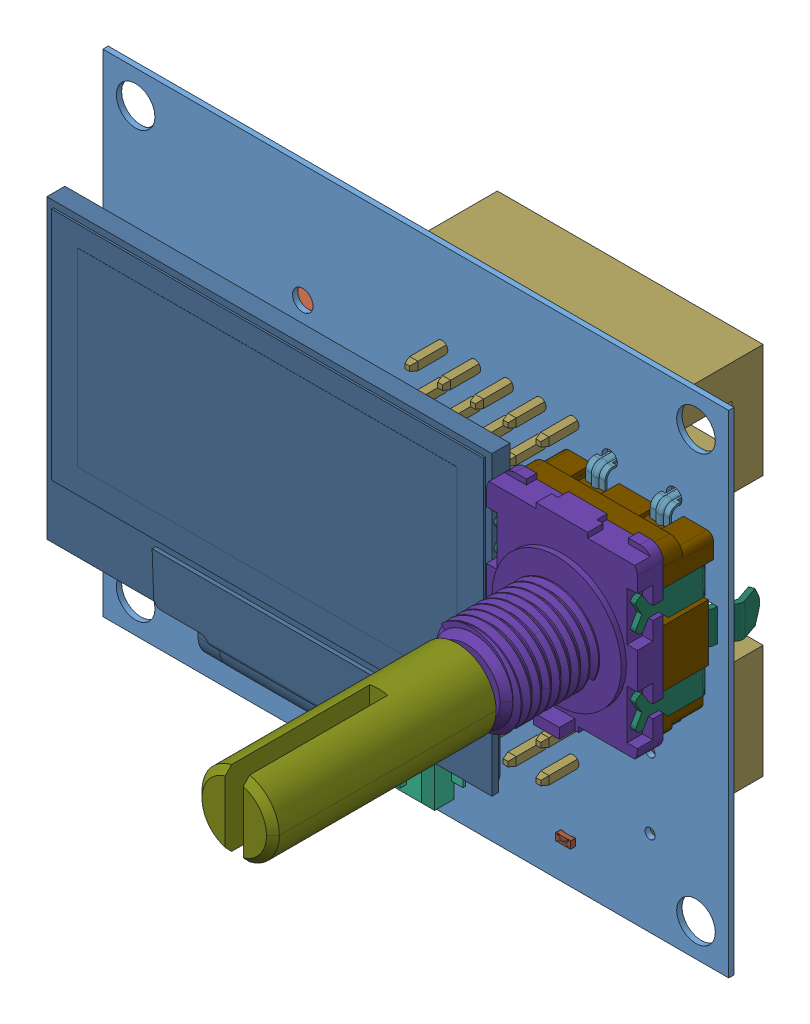
SolidWorks assembly PCB2, configuration 默认. Lengths in mm.
Overall size (48.51 38.1 41.11).
81 component instances, 19 part files, 0 mates.
Components (placement in the parent):
- PCB2.step-1: PCB2.step [默认] at origin size (48.51 38.1 41.11)
  - Board.step-1: Board.step [默认] at origin size (48.51 38.1 0.41)
    - Open CASCADE STEP translator 6.8 1.1.1.step-1: Open CASCADE STEP translator 6.8 1.1.1.step [默认] at (0 0 -0.4115) size (48.51 38.1 0.41)
  - U2.step-1: U2.step [默认] at origin size (18.85 27.3 3.6)
    - User_Library-SDCARD.step-1: User_Library-SDCARD.step [默认] at (12.9551 16.5451 -0.4115) x (0 1 0) z (0 0 -1) size (27.3 18 3)
      - Pad002.step-1: Pad002.step [默认] at origin size (27.3 18 3)
    - User_Library-Micro_SD_Socket_Push-push.step-1: User_Library-Micro_SD_Socket_Push-push.step [默认] at (12.0551 14.7951 -0.4115) x (0 -1 0) z (1 0 0) size (16.1 2.45 15)
  - P1.step-1: P1.step [默认] at origin size (11.4 4.2 4.75)
    - 533980571.step-1: 533980571.step [默认] at (8.8749 -0.3421 -4.2115) x (1 0 0) z (0 1 0) size (11.4 4.75 4.2)
      - Open CASCADE STEP translator 6.8 1.3.1.1.step-1: Open CASCADE STEP translator 6.8 1.3.1.1.step [默认] at origin size (11.4 4.75 4.2)
      - Open CASCADE STEP translator 6.8 1.3.1.2.step-1: Open CASCADE STEP translator 6.8 1.3.1.2.step [默认] at origin
  - C16.step-1: C16.step [默认] at origin size (1 0.6 0.2)
    - 0402_SMD_Capacitor.step-1: 0402_SMD_Capacitor.step [默认] at (42.1466 25.527 -0.4115) x (-1 0 0) z (0 -1 0) size (1 0.2 0.6)
  - B1.step-1: B1.step [默认] at origin size (7.9 3.65 2.5)
    - User_Library-smd_buttonm_8mm.step-1: User_Library-smd_buttonm_8mm.step [默认] at (21.6225 0.6317 0) x (-1 0 0) z (0 1 0) size (7.9 2.5 3.65)
  - C15.step-1: C15.step [默认] at origin size (0.6 1 0.2)
    - 0402_SMD_Capacitor.step-1: 0402_SMD_Capacitor.step [默认] at (18.923 16.0194 -0.4115) x (0 1 0) z (-1 0 0) size (1 0.2 0.6)
  - C14.step-1: C14.step [默认] at origin size (0.6 1 0.2)
    - 0402_SMD_Capacitor.step-1: 0402_SMD_Capacitor.step [默认] at (17.653 16.0194 -0.4115) x (0 1 0) z (-1 0 0) size (1 0.2 0.6)
  - C13.step-1: C13.step [默认] at origin size (1.68 3.4 1.71)
    - User_Library-AVX_ACASE.step-1: User_Library-AVX_ACASE.step [默认] at (9.3979 32.0039 -0.4115) x (0 -1 0) z (0 0 -1) size (3.4 1.68 1.71)
  - C12.step-1: C12.step [默认] at origin size (1.68 3.4 1.71)
    - User_Library-AVX_ACASE.step-1: User_Library-AVX_ACASE.step [默认] at (17.2719 31.9169 -0.4115) x (0 -1 0) z (0 0 -1) size (3.4 1.68 1.71)
  - C11.step-1: C11.step [默认] at origin size (1 0.6 0.2)
    - 0402_SMD_Capacitor.step-1: 0402_SMD_Capacitor.step [默认] at (21.8614 0.635 -0.4115) x (1 0 0) z (0 1 0) size (1 0.2 0.6)
  - C10.step-1: C10.step [默认] at origin size (1 0.6 0.2)
    - 0402_SMD_Capacitor.step-1: 0402_SMD_Capacitor.step [默认] at (22.9604 22.479 -0.4115) x (1 0 0) z (0 1 0) size (1 0.2 0.6)
  - U4.step-1: U4.step [默认] at origin size (3 3 1.3)
    - SOT-23.step-1: SOT-23.step [默认] at (12.5729 32.1311 -0.4115) x (0 -1 0) z (1 0 0) size (3 1.3 3)
  - U3.step-1: U3.step [默认] at origin size (9.9 6 1.75)
    - SOIC16P127_990X600X175L60X40N.step-1: SOIC16P127_990X600X175L60X40N.step [默认] at (27.813 17.944 -0.4115) x (1 0 0) z (0 0 -1) size (9.9 6 1.75)
  - U1.step-1: U1.step [默认] at origin size (34.61 26.11 4.75)
    - User_Library-OLED-1_3C.step-1: User_Library-OLED-1_3C.step [默认] at (14.8341 14.2411 4) x (1 0 0) z (0 -1 0) size (34.61 4.75 26.11)
  - R6.step-1: R6.step [默认] at origin size (1.15 0.55 0.41)
    - User_Library-RES_1005-0402.step-1: User_Library-RES_1005-0402.step [默认] at (23.876 -0.635 -0.4115) x (-1 0 0) z (0 -1 0) size (1.15 0.41 0.55)
  - R5.step-1: R5.step [默认] at origin size (1.15 0.55 0.41)
    - User_Library-RES_1005-0402.step-1: User_Library-RES_1005-0402.step [默认] at (23.876 2.032 -0.4115) x (-1 0 0) z (0 -1 0) size (1.15 0.41 0.55)
  - R4.step-1: R4.step [默认] at origin size (1.15 0.55 0.41)
    - User_Library-RES_1005-0402.step-1: User_Library-RES_1005-0402.step [默认] at (21.844 2.032 -0.4115) x (-1 0 0) z (0 -1 0) size (1.15 0.41 0.55)
  - R3.step-1: R3.step [默认] at origin size (1.15 0.55 0.41)
    - User_Library-RES_1005-0402.step-1: User_Library-RES_1005-0402.step [默认] at (33.528 0.635 0) x (1 0 0) z (0 -1 0) size (1.15 0.41 0.55)
  - R2.step-1: R2.step [默认] at origin size (1.15 0.55 0.41)
    - User_Library-RES_1005-0402.step-1: User_Library-RES_1005-0402.step [默认] at (21.844 21.336 -0.4115) x (-1 0 0) z (0 -1 0) size (1.15 0.41 0.55)
  - R1.step-1: R1.step [默认] at origin size (1.15 0.55 0.41)
    - User_Library-RES_1005-0402.step-1: User_Library-RES_1005-0402.step [默认] at (33.0667 0.254 -0.4115) x (1 0 0) z (0 1 0) size (1.15 0.41 0.55)
  - Q1.step-1: Q1.step [默认] at origin size (3 3 1.3)
    - SOT-23.step-1: SOT-23.step [默认] at (36.5759 0.2539 -0.4115) x (1 0 0) z (0 1 0) size (3 1.3 3)
  - EXP2.step-1: EXP2.step [默认] at origin size (20.6 8.8 12.2)
    - User_Library-BoxHeader_2R5W_254P_00D.step-1: User_Library-BoxHeader_2R5W_254P_00D.step [默认] at (28.8291 27.412 -0.4115) x (1 0 0) z (0 1 0) size (20.6 12.2 8.8)
  - EXP1.step-1: EXP1.step [默认] at origin size (20.6 8.8 12.2)
    - User_Library-BoxHeader_2R5W_254P_00D.step-1: User_Library-BoxHeader_2R5W_254P_00D.step [默认] at (28.8291 7.219 -0.4115) x (1 0 0) z (0 1 0) size (20.6 12.2 8.8)
  - EC1.step-1: EC1.step [默认] at origin size (13.1 15.13 35.07)
    - User_Library-EC11B15244.step-1: User_Library-EC11B15244.step [默认] at (39.2429 20.7079 0) x (-1 0 0) z (0 0 1) size (13.1 15.13 35.07)
      - Pins.step-1: Pins.step [默认] at (0 0 6.6326) size (13.1 14.95 9.45)
        - Imported.step-1: Imported.step [默认] at (-2.5 7.575 -10.2243) x (0 -1 0) z (0 0 1) size (2.34 1.5 6.65)
        - Imported.step-2: Imported.step [默认] at (0 7.575 -10.2243) x (0 -1 0) z (0 0 1) size (2.34 1.5 6.65)
        - Imported.step-3: Imported.step [默认] at (2.5 7.575 -10.2243) x (0 -1 0) z (0 0 1) size (2.34 1.5 6.65)
        - Pin.step-1: Pin.step [默认] at (-2.5 -7.075 -10.2243) x (0 1 0) z (0 0 1) size (2.15 1.5 4.73)
        - Pin.step-2: Pin.step [默认] at (2.5 -7.075 -10.2243) x (0 1 0) z (0 0 1) size (2.15 1.5 4.73)
        - Sheet_Metal_Part53.step-1: Sheet_Metal_Part53.step [默认] at (-24.7094 3.8245 8.4125) size (13.1 9.9 9.18)
      - Shaft.step-1: Shaft.step [默认] at (0 0 13.6) size (6 6 18)
      - MetalBody.step-1: MetalBody.step [默认] at (0 0 3.443) size (11.7 13.8 9.4)
      - PlasticBody.step-1: PlasticBody.step [默认] at (-0.85 -0.6436 6.5892) size (11.7 13.3 3.9)
  - C9.step-1: C9.step [默认] at origin size (0.6 1 0.2)
    - 0402_SMD_Capacitor.step-1: 0402_SMD_Capacitor.step [默认] at (7.747 32.1484 -0.4115) x (0 1 0) z (-1 0 0) size (1 0.2 0.6)
  - C8.step-1: C8.step [默认] at origin size (0.6 1 0.2)
    - 0402_SMD_Capacitor.step-1: 0402_SMD_Capacitor.step [默认] at (15.367 32.0654 -0.4115) x (0 1 0) z (-1 0 0) size (1 0.2 0.6)
  - C7.step-1: C7.step [默认] at origin size (1 0.6 0.2)
    - 0402_SMD_Capacitor.step-1: 0402_SMD_Capacitor.step [默认] at (23.9856 13.589 -0.4115) x (-1 0 0) z (0 -1 0) size (1 0.2 0.6)
  - C6.step-1: C6.step [默认] at origin size (1 0.6 0.2)
    - 0402_SMD_Capacitor.step-1: 0402_SMD_Capacitor.step [默认] at (23.9856 12.446 -0.4115) x (-1 0 0) z (0 -1 0) size (1 0.2 0.6)
  - C5.step-1: C5.step [默认] at origin size (1 0.6 0.2)
    - 0402_SMD_Capacitor.step-1: 0402_SMD_Capacitor.step [默认] at (21.9884 13.589 -0.4115) x (1 0 0) z (0 1 0) size (1 0.2 0.6)
  - C4.step-1: C4.step [默认] at origin size (1 0.6 0.2)
    - 0402_SMD_Capacitor.step-1: 0402_SMD_Capacitor.step [默认] at (6.8944 20.4534 0) x (1 0 0) z (0 -1 0) size (1 0.2 0.6)
  - C3.step-1: C3.step [默认] at origin size (1 0.6 0.2)
    - 0402_SMD_Capacitor.step-1: 0402_SMD_Capacitor.step [默认] at (4.9303 20.4464 0) x (1 0 0) z (0 -1 0) size (1 0.2 0.6)
  - C2.step-1: C2.step [默认] at origin size (1 0.6 0.2)
    - 0402_SMD_Capacitor.step-1: 0402_SMD_Capacitor.step [默认] at (10.7776 20.447 0) x (-1 0 0) z (0 1 0) size (1 0.2 0.6)
  - C1.step-1: C1.step [默认] at origin size (1 0.6 0.2)
    - 0402_SMD_Capacitor.step-1: 0402_SMD_Capacitor.step [默认] at (8.7957 20.4464 0) x (-1 0 0) z (0 1 0) size (1 0.2 0.6)
